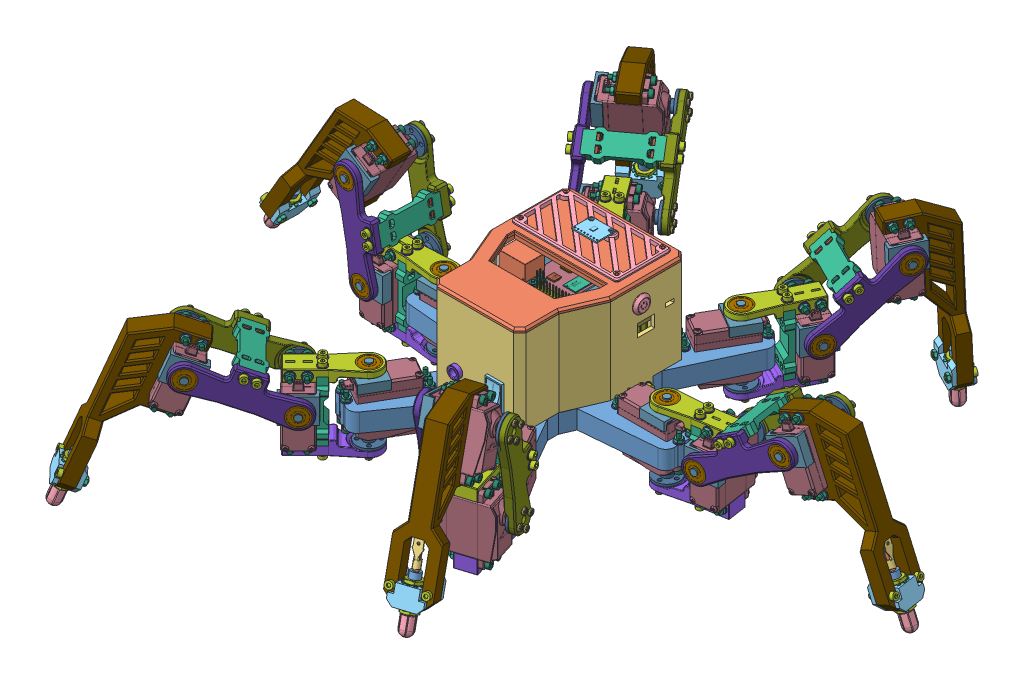
SolidWorks assembly HEXUMI_DSSERVO, configuration Default. Lengths in mm.
Overall size (517.79 216.76 502.75).
850 component instances, 62 part files, 169 mates.
Components (placement in the parent):
- BODY_ASM-1: BODY_ASM [Default] at origin size (216.8 93.6 230.48)
  - MAIN_FRAME-1: MAIN_FRAME [Default] at origin size (216.8 15 230.48)
  - LID-1: LID [Default] at (-25.1298 69 304.4932) x (1 0 0) z (0 1 0) size (97 123 7)
  - MID CASE-1: MID CASE [Default] at origin size (97 79 123)
  - ON_SWITCH-1: ON_SWITCH [Default] at (33.5 56 5) x (0 0.109318 -0.994007) z (0 -0.994007 -0.109318) size (13.7 18.1 13.7)
  - POWER_SWITCH-1: POWER_SWITCH [Default] at (16.5 19.5 76) x (0 -1 0) z (-1 0 0) size (20.5 20.17 13.5)
  - M3_HEX_NUT-1: M3_HEX_NUT [Default] at (-35 -5 0) x (0 -0.865861 0.500284) z (0 0.500284 0.865861) size (6.98 2.4 5.5)
  - M3_STEEL_HEX_BOLT_16MM-1: M3_STEEL_HEX_BOLT_16MM [Default] at (0 -5 -36.5) x (0.06898 0.997618 0) z (0.997618 -0.06898 0) size (5.68 19 5.68)
  - M3_WASHER-1: M3_WASHER [Default] at (-49 -5 0) x (0 -0.533756 -0.845639) z (0 -0.845639 0.533756) size (7 0.5 7)
  - M3_HEX_NUT-2: M3_HEX_NUT [Default] at (0 -5 -20.5) x (0.938223 0.346031 0) z (0.346031 -0.938223 0) size (6.98 2.4 5.5)
  - M3_HEX_NUT-3: M3_HEX_NUT [Default] at (0 -5 75.1) x (0.997389 -0.072217 0) z (-0.072217 -0.997389 0) size (6.98 2.4 5.5)
  - M3_HEX_NUT-4: M3_HEX_NUT [Default] at (32.6 -5 0) x (0 -0.520946 -0.85359) z (0 -0.85359 0.520946) size (6.98 2.4 5.5)
  - M3_STEEL_HEX_BOLT_16MM-2: M3_STEEL_HEX_BOLT_16MM [Default] at (-52 -5 0) x (0 -0.536208 -0.844086) z (0 -0.844086 0.536208) size (5.68 19 5.68)
  - M3_STEEL_HEX_BOLT_16MM-3: M3_STEEL_HEX_BOLT_16MM [Default] at (52 -5 0) x (0 0.249062 -0.968488) z (0 0.968488 0.249062) size (5.68 19 5.68)
  - M3_STEEL_HEX_BOLT_16MM-4: M3_STEEL_HEX_BOLT_16MM [Default] at (0 -5 93.5) x (-0.010084 0.999949 0) z (-0.999949 -0.010084 0) size (5.68 19 5.68)
  - M3_WASHER-2: M3_WASHER [Default] at (48.5 -5 0) x (0 -0.753455 -0.657499) z (0 -0.657499 0.753455) size (7 0.5 7)
  - M3_WASHER-3: M3_WASHER [Default] at (0 -5 90.5) x (0.583401 0.812184 0) z (-0.812184 0.583401 0) size (7 0.5 7)
  - M3_WASHER-4: M3_WASHER [Default] at (0 -5 -33) x (0.7999 0.600134 0) z (-0.600134 0.7999 0) size (7 0.5 7)
  - INNER_FRAME_ASM_BRASS-1: INNER_FRAME_ASM_BRASS [Default] at (0 3.6 0) size (89.3 62.14 116.59)
    - power frame R-1: power frame R [Default] at origin size (85 4 113)
    - M2.5_STEEL_HEX_NUT-1: M2.5_STEEL_HEX_NUT [Default] at (39 -1.8 -24.5) x (-0.53176 0 -0.846895) z (0.846895 0 -0.53176) size (6.22 1.8 4.9)
    - M2.5_STEEL_HEX_NUT-2: M2.5_STEEL_HEX_NUT [Default] at (-28.3 -1.8 82.3) x (-0.926596 0 0.376059) z (-0.376059 0 -0.926596) size (6.22 1.8 4.9)
    - M2.5_STEEL_HEX_NUT-3: M2.5_STEEL_HEX_NUT [Default] at (28.3 -1.8 82.3) x (-0.90596 0 -0.423363) z (0.423363 0 -0.90596) size (6.22 1.8 4.9)
    - M2.5_STEEL_HEX_NUT-4: M2.5_STEEL_HEX_NUT [Default] at (-19 -1.8 -24.5) x (0.987479 0 -0.157753) z (0.157753 0 0.987479) size (6.22 1.8 4.9)
    - M2.5_BRASS_SPACER_20MM-1: M2.5_BRASS_SPACER_20MM [Default] at (28.3 16.5 82.3) x (0.147579 0 -0.98905) z (0.98905 0 0.147579) size (5.43 25 4.7)
    - M2.5_BRASS_SPACER_20MM-2: M2.5_BRASS_SPACER_20MM [Default] at (-19 16.5 -24.5) x (0.999419 0 0.034097) z (-0.034097 0 0.999419) size (5.43 25 4.7)
    - M2.5_BRASS_SPACER_20MM-3: M2.5_BRASS_SPACER_20MM [Default] at (-28.3 16.5 82.3) x (0.586169 0 0.810189) z (-0.810189 0 0.586169) size (5.43 25 4.7)
    - M2.5_BRASS_SPACER_20MM-4: M2.5_BRASS_SPACER_20MM [Default] at (39 16.5 -24.5) x (0.00416 0 -0.999991) z (0.999991 0 0.00416) size (5.43 25 4.7)
    - RPi FRAME-1: RPi FRAME [Default] at (0 30.8 0) size (85 4 113)
    - M2.5_STEEL_HEX_NUT-9: M2.5_STEEL_HEX_NUT [Default] at (39 34.8 -24.5) x (0.941663 0 -0.336557) z (0.336557 0 0.941663) size (6.22 1.8 4.9)
    - M2.5_STEEL_HEX_NUT-10: M2.5_STEEL_HEX_NUT [Default] at (28.3 34.8 82.3) x (-0.299428 0 -0.954119) z (0.954119 0 -0.299428) size (6.22 1.8 4.9)
    - M2.5_STEEL_HEX_NUT-11: M2.5_STEEL_HEX_NUT [Default] at (28.3 34.8 45.7) x (-0.609973 0 0.792422) z (-0.792422 0 -0.609973) size (6.22 1.8 4.9)
    - M2.5_STEEL_HEX_NUT-12: M2.5_STEEL_HEX_NUT [Default] at (39 34.8 24.5) x (-0.398443 0 0.917193) z (-0.917193 0 -0.398443) size (6.22 1.8 4.9)
    - M2.5_STEEL_HEX_NUT-13: M2.5_STEEL_HEX_NUT [Default] at (-19 34.8 -24.5) x (-0.889727 0 0.456493) z (-0.456493 0 -0.889727) size (6.22 1.8 4.9)
    - M2.5_STEEL_HEX_NUT-14: M2.5_STEEL_HEX_NUT [Default] at (-19 34.8 24.5) x (-0.550521 0 -0.834821) z (0.834821 0 -0.550521) size (6.22 1.8 4.9)
    - M2.5_STEEL_HEX_NUT-15: M2.5_STEEL_HEX_NUT [Default] at (-28.3 34.8 82.3) x (-0.427939 0 0.903808) z (-0.903808 0 -0.427939) size (6.22 1.8 4.9)
    - M2.5_STEEL_HEX_NUT-16: M2.5_STEEL_HEX_NUT [Default] at (-28.3 34.8 45.7) x (-0.613101 0 -0.790005) z (0.790005 0 -0.613101) size (6.22 1.8 4.9)
    - Raspberry Pi 4 Model B-1: Raspberry Pi 4 Model B [Default] at (0 39.19 0) x (-1 0 0) z (0 0 -1) size (88.99 19.9 58.4)
      - PCB, RPi4ModelB-1: PCB, RPi4ModelB [Default] at origin size (85 1.6 56)
      - Broadcom BCM2711B0 CPU, RPi4ModelB-1: Broadcom BCM2711B0 CPU, RPi4ModelB [Default] at (-13.25 0.8 -4.5) size (15 2.3 15)
      - 2.54 mm DUPONT MALE PIN HEADER, POE, 2X2, RPi4ModelB-1: 2.54 mm DUPONT MALE PIN HEADER, POE, 2X2, RPi4ModelB [Default] at (19 0.8 -18.5) size (5.08 11.3 5.08)
      - 2.54 mm DUPONT MALE PIN HEADER, IO, 2X20, RPi4ModelB-1: 2.54 mm DUPONT MALE PIN HEADER, IO, 2X20, RPi4ModelB [Default] at (-10 0.8 -24.5) size (50.8 11.3 5.08)
      - Camera Connector, RPi4ModelB-1: Camera Connector, RPi4ModelB [Default] at (4 0.8 16.5) x (0 0 -1) z (1 0 0) size (22.4 5.68 5.07)
      - Microphone Plug, RPi4ModelB-1: Microphone Plug, RPi4ModelB [Default] at (11.5 0.8 21.65) size (7.23 7.55 15)
      - Display Connector, RPi4ModelB-1: Display Connector, RPi4ModelB [Default] at (-38.5 0.8 0) x (0 0 1) z (-1 0 0) size (22.4 5.68 5.07)
      - Gigabit Ethernet Port, RPi4ModelB-1: Gigabit Ethernet Port, RPi4ModelB [Default] at (45.5 7.55 -17.75) x (0 0 -1) z (1 0 0) size (16.2 17.24 21.64)
      - Female Micro HDMI Connector, RPi4ModelB-2: Female Micro HDMI Connector, RPi4ModelB [Default] at (-3 0.8 27.3875) size (6.5 3.51 7.5)
      - Female Micro HDMI Connector, RPi4ModelB-3: Female Micro HDMI Connector, RPi4ModelB [Default] at (-16.5 0.8 27.3875) size (6.5 3.51 7.5)
      - Female USB Type C Connector, RPi4ModelB-1: Female USB Type C Connector, RPi4ModelB [Default] at (-31.3 0.8 26.5419) size (8.94 3.96 7.9)
      - 2X USB3.0 PORTS, RPi4ModelB-2: 2X USB3.0 PORTS, RPi4ModelB [Default] at (37.07 0.8 1) size (17.47 19.41 15.68)
      - 91D77 D9WHV 778K, 4 GB LPDDR4 SDRAM, RPi4ModelB-1: 91D77 D9WHV 778K, 4 GB LPDDR4 SDRAM, RPi4ModelB [Default] at (2.25 0.8 -4.5) size (10 0.8 14.5)
      - Cypress CYW43455 Wireless Module Cover, RPi4ModelB-1: Cypress CYW43455 Wireless Module Cover, RPi4ModelB [Default] at (-30.5 0.8 -14.5) size (11 1.6 13)
      - SD Card Slot, RPi4ModelB-1: SD Card Slot, RPi4ModelB [Default] at (-35.3 -0.8 0) x (0 0 -1) z (-1 0 0) size (11.95 1.45 11.4)
      - VIA VL805 PCIe USB 3.0 controller, RPi4ModelB-1: VIA VL805 PCIe USB 3.0 controller, RPi4ModelB [Default] at (17.5 0.8 4) size (8.8 0.8 8.8)
      - 2X USB2.0 PORTS, RPi4ModelB-1: 2X USB2.0 PORTS, RPi4ModelB [Default] at (37.065 0.65 19) size (17.87 19.16 15.33)
      - Broadcom BCM54213PE Gigabit Ethernet Transceiver, RPi4ModelB-1: Broadcom BCM54213PE Gigabit Ethernet Transceiver, RPi4ModelB [Default] at (16.5 0.8 -10) size (6.8 1 6.8)
      - MxL7704 Universal PMIC, RPi4ModelB-1: MxL7704 Universal PMIC, RPi4ModelB [Default] at (-32.5 0.8 16) size (5.4 0.8 5.4)
    - M2.5_STEEL_TRI_BOLT_20MM-1: M2.5_STEEL_TRI_BOLT_20MM [Default] at (39 43.28 -24.5) x (0.010584 0 0.999944) z (0.999944 0 -0.010584) size (4.7 20 4.7)
    - M2.5_STEEL_HEX_NUT-17: M2.5_STEEL_HEX_NUT [Default] at (39 39.98 24.5) x (0.999676 0 0.025448) z (-0.025448 0 0.999676) size (6.22 1.8 4.9)
    - M2.5_STEEL_HEX_NUT-18: M2.5_STEEL_HEX_NUT [Default] at (-28.3 38.2 82.3) x (0.982697 0 -0.185221) z (0.185221 0 0.982697) size (6.22 1.8 4.9)
    - M2.5_STEEL_HEX_NUT-19: M2.5_STEEL_HEX_NUT [Default] at (28.3 38.2 82.3) size (6.22 1.8 4.9)
    - M2.5_STEEL_HEX_NUT-20: M2.5_STEEL_HEX_NUT [Default] at (28.3 38.2 45.7) size (6.22 1.8 4.9)
    - M2.5_STEEL_HEX_NUT-21: M2.5_STEEL_HEX_NUT [Default] at (-28.3 38.2 45.7) size (6.22 1.8 4.9)
    - M2.5_STEEL_HEX_NUT-22: M2.5_STEEL_HEX_NUT [Default] at (-19 39.98 24.5) x (0.99488 0 -0.101065) z (0.101065 0 0.99488) size (6.22 1.8 4.9)
    - M2.5_STEEL_HEX_NUT-23: M2.5_STEEL_HEX_NUT [Default] at (-19 39.98 -24.5) x (0.853732 0 0.520713) z (-0.520713 0 0.853732) size (6.22 1.8 4.9)
    - M2.5_STEEL_HEX_NUT-24: M2.5_STEEL_HEX_NUT [Default] at (39 39.98 -24.5) x (0.977205 0 0.212296) z (-0.212296 0 0.977205) size (6.22 1.8 4.9)
    - M2.5_STEEL_TRI_BOLT_20MM-2: M2.5_STEEL_TRI_BOLT_20MM [Default] at (28.3 41.5 82.3) x (0.000016 0 1) z (1 0 -0.000016) size (4.7 20 4.7)
    - M2.5_STEEL_TRI_BOLT_20MM-3: M2.5_STEEL_TRI_BOLT_20MM [Default] at (-28.3 41.5 82.3) x (0.000016 0 1) z (1 0 -0.000016) size (4.7 20 4.7)
    - M2.5_STEEL_TRI_BOLT_20MM-4: M2.5_STEEL_TRI_BOLT_20MM [Default] at (-19 43.28 -24.5) x (0.000016 0 1) z (1 0 -0.000016) size (4.7 20 4.7)
    - SERVO_2040-1: SERVO_2040 [Default] at (0 36.6 64) x (-1 0 0) z (0 0 -1) size (63.5 10.6 42)
    - M2.5_NYLON_BOLT-1: M2.5_NYLON_BOLT [Default] at (-28.3 41.5 45.7) x (0.149804 0 0.988716) z (0.988716 0 -0.149804) size (4.7 15 4.7)
    - M2.5_NYLON_BOLT-2: M2.5_NYLON_BOLT [Default] at (39 43.28 24.5) x (0.149804 0 0.988716) z (0.988716 0 -0.149804) size (4.7 15 4.7)
    - M2.5_NYLON_BOLT-3: M2.5_NYLON_BOLT [Default] at (28.3 41.5 45.7) x (0.149804 0 0.988716) z (0.988716 0 -0.149804) size (4.7 15 4.7)
    - M2.5_NYLON_BOLT-4: M2.5_NYLON_BOLT [Default] at (-19 43.28 24.5) x (0.05042 0 -0.998728) z (-0.998728 0 -0.05042) size (4.7 15 4.7)
    - M2.5_STEEL_HEX_NUT-25: M2.5_STEEL_HEX_NUT [Default] at (28.3 29 45.7) size (6.22 1.8 4.9)
    - M2.5_STEEL_HEX_NUT-26: M2.5_STEEL_HEX_NUT [Default] at (-28.3 29 45.7) x (0.960779 0 0.277315) z (-0.277315 0 0.960779) size (6.22 1.8 4.9)
    - M2.5_STEEL_HEX_NUT-27: M2.5_STEEL_HEX_NUT [Default] at (-19 29 24.5) x (0.999926 0 0.01217) z (-0.01217 0 0.999926) size (6.22 1.8 4.9)
    - M2.5_STEEL_HEX_NUT-28: M2.5_STEEL_HEX_NUT [Default] at (39 29 24.5) x (0.999999 0 -0.001638) z (0.001638 0 0.999999) size (6.22 1.8 4.9)
    - 7V_BUCK-1: 7V_BUCK [Default] at (13.575 6 12.675) x (0 0 1) z (-1 0 0) size (65.3 21.55 50.1)
    - 3.3V_RELAY-1: 3.3V_RELAY [Default] at (-21.55 5.2 16.3) x (0 0 1) z (-1 0 0) size (70 18 17)
    - M2.5_NYLON_HEX_NUT-1: M2.5_NYLON_HEX_NUT [Default] at (0.65 -2 41.35) size (5.66 2 4.9)
    - M2.5_NYLON_HEX_NUT-2: M2.5_NYLON_HEX_NUT [Default] at (26.5 4 -16) size (5.66 2 4.9)
    - M2.5_NYLON_HEX_NUT-3: M2.5_NYLON_HEX_NUT [Default] at (0.65 4 41.35) size (5.66 2 4.9)
    - M2.5_NYLON_HEX_NUT-4: M2.5_NYLON_HEX_NUT [Default] at (26.5 -2 41.35) size (5.66 2 4.9)
    - M2.5_NYLON_HEX_NUT-5: M2.5_NYLON_HEX_NUT [Default] at (26.5 4 41.35) size (5.66 2 4.9)
    - M2.5_NYLON_HEX_NUT-6: M2.5_NYLON_HEX_NUT [Default] at (0.65 4 -16) size (5.66 2 4.9)
    - M2.5_NYLON_HEX_NUT-7: M2.5_NYLON_HEX_NUT [Default] at (0.65 -2 -16) size (5.66 2 4.9)
    - M2.5_NYLON_HEX_NUT-8: M2.5_NYLON_HEX_NUT [Default] at (26.5 -2 -16) size (5.66 2 4.9)
    - M2_NYLON_HEX_NUT-1: M2_NYLON_HEX_NUT [Default] at (-27.75 4 -16) size (4.39 1.2 3.8)
    - M2_NYLON_HEX_NUT-2: M2_NYLON_HEX_NUT [Default] at (-27.75 -1.2 48.6) x (0.996977 0 0.0777) z (-0.0777 0 0.996977) size (4.39 1.2 3.8)
    - M2_NYLON_HEX_NUT-3: M2_NYLON_HEX_NUT [Default] at (-15.35 4 -16) size (4.39 1.2 3.8)
    - M2_NYLON_HEX_NUT-5: M2_NYLON_HEX_NUT [Default] at (-15.35 -1.2 48.6) size (4.39 1.2 3.8)
    - M2_NYLON_HEX_NUT-6: M2_NYLON_HEX_NUT [Default] at (-15.35 -1.2 -16) x (-0.796408 0 -0.604759) z (0.604759 0 -0.796408) size (4.39 1.2 3.8)
    - M2_NYLON_HEX_NUT-8: M2_NYLON_HEX_NUT [Default] at (-27.75 -1.2 -16) x (-0.852858 0 0.522143) z (-0.522143 0 -0.852858) size (4.39 1.2 3.8)
    - M2_NYLON_HEX_NUT-9: M2_NYLON_HEX_NUT [Default] at (-27.75 4 48.6) size (4.39 1.2 3.8)
    - M2_NYLON_HEX_NUT-10: M2_NYLON_HEX_NUT [Default] at (-15.35 4 48.6) size (4.39 1.2 3.8)
    - M2.5_STEEL_HEX_NUT-29: M2.5_STEEL_HEX_NUT [Default] at (-28.3 29 82.3) x (-0.398443 0 0.917193) z (-0.917193 0 -0.398443) size (6.22 1.8 4.9)
    - M2.5_STEEL_HEX_NUT-30: M2.5_STEEL_HEX_NUT [Default] at (-19 29 -24.5) x (-0.398443 0 0.917193) z (-0.917193 0 -0.398443) size (6.22 1.8 4.9)
    - M2.5_STEEL_HEX_NUT-31: M2.5_STEEL_HEX_NUT [Default] at (28.3 29 82.3) x (-0.187174 0 0.982327) z (-0.982327 0 -0.187174) size (6.22 1.8 4.9)
    - M2.5_STEEL_HEX_NUT-32: M2.5_STEEL_HEX_NUT [Default] at (39 29 -24.5) x (-0.432758 0 0.90151) z (-0.90151 0 -0.432758) size (6.22 1.8 4.9)
    - M2.5_NYLON_BOLT-5: M2.5_NYLON_BOLT [Default] at (26.5 9.05 41.35) x (0.298465 0 -0.954421) z (-0.954421 0 -0.298465) size (4.7 15 4.7)
    - M2.5_NYLON_BOLT-6: M2.5_NYLON_BOLT [Default] at (0.65 9.05 -16) x (0.311969 0 -0.950092) z (-0.950092 0 -0.311969) size (4.7 15 4.7)
    - M2.5_NYLON_BOLT-7: M2.5_NYLON_BOLT [Default] at (26.5 9.05 -16) x (0.298465 0 -0.954421) z (-0.954421 0 -0.298465) size (4.7 15 4.7)
    - M2.5_NYLON_BOLT-8: M2.5_NYLON_BOLT [Default] at (0.65 9.05 41.35) x (0.298465 0 -0.954421) z (-0.954421 0 -0.298465) size (4.7 15 4.7)
    - M2_NYLON_BOLT-1: M2_NYLON_BOLT [Default] at (-27.75 7.8 48.6) x (-0.556663 0 -0.830738) z (-0.830738 0 0.556663) size (3.8 10 3.8)
    - M2_NYLON_BOLT-2: M2_NYLON_BOLT [Default] at (-15.35 7.8 48.6) x (-0.518121 0 -0.855307) z (-0.855307 0 0.518121) size (3.8 10 3.8)
    - M2_NYLON_BOLT-3: M2_NYLON_BOLT [Default] at (-27.75 7.8 -16) x (-0.556663 0 -0.830738) z (-0.830738 0 0.556663) size (3.8 10 3.8)
    - M2_NYLON_BOLT-4: M2_NYLON_BOLT [Default] at (-15.35 7.8 -16) x (-0.556663 0 -0.830738) z (-0.830738 0 0.556663) size (3.8 10 3.8)
    - 5v_buck-1: 5v_buck [Default] at (19 31.6 -14) x (1 0 0) z (0 0 -1) size (33 7.8 28.5)
    - M2_NYLON_BOLT-5: M2_NYLON_BOLT [Default] at (32.95 35.9 -15.7) x (0.89104 0 -0.453925) z (-0.453925 0 -0.89104) size (3.8 10 3.8)
    - M2_NYLON_BOLT-6: M2_NYLON_BOLT [Default] at (5.05 35.9 -2.5) x (0.891706 0 -0.452615) z (-0.452615 0 -0.891706) size (3.8 10 3.8)
    - M2_NYLON_BOLT-7: M2_NYLON_BOLT [Default] at (5.05 35.9 -15.7) x (0.896031 0 -0.443992) z (-0.443992 0 -0.896031) size (3.8 10 3.8)
    - M2_NYLON_BOLT-8: M2_NYLON_BOLT [Default] at (32.95 35.9 -2.5) x (0.891706 0 -0.452615) z (-0.452615 0 -0.891706) size (3.8 10 3.8)
    - M2_NYLON_HEX_NUT-11: M2_NYLON_HEX_NUT [Default] at (32.95 31.6 -2.5) size (4.39 1.2 3.8)
    - M2_NYLON_HEX_NUT-12: M2_NYLON_HEX_NUT [Default] at (32.95 31.6 -15.7) size (4.39 1.2 3.8)
    - M2_NYLON_HEX_NUT-13: M2_NYLON_HEX_NUT [Default] at (5.05 31.6 -2.5) size (4.39 1.2 3.8)
    - M2_NYLON_HEX_NUT-14: M2_NYLON_HEX_NUT [Default] at (5.05 31.6 -15.7) size (4.39 1.2 3.8)
    - M2_NYLON_HEX_NUT-15: M2_NYLON_HEX_NUT [Default] at (32.95 28.9 -15.7) size (4.39 1.2 3.8)
    - M2_NYLON_HEX_NUT-16: M2_NYLON_HEX_NUT [Default] at (5.05 28.9 -15.7) size (4.39 1.2 3.8)
    - M2_NYLON_HEX_NUT-17: M2_NYLON_HEX_NUT [Default] at (32.95 28.9 -2.5) size (4.39 1.2 3.8)
    - M2_NYLON_HEX_NUT-18: M2_NYLON_HEX_NUT [Default] at (5.05 28.9 -2.5) size (4.39 1.2 3.8)
    - M2.5_STEEL_HEX_NUT-33: M2.5_STEEL_HEX_NUT [Default] at (-19 36.6 -24.5) x (-0.398443 0 0.917193) z (-0.917193 0 -0.398443) size (6.22 1.8 4.9)
    - M2.5_STEEL_HEX_NUT-34: M2.5_STEEL_HEX_NUT [Default] at (39 36.6 24.5) x (-0.398443 0 0.917193) z (-0.917193 0 -0.398443) size (6.22 1.8 4.9)
    - M2.5_STEEL_HEX_NUT-35: M2.5_STEEL_HEX_NUT [Default] at (-19 36.6 24.5) x (-0.398443 0 0.917193) z (-0.917193 0 -0.398443) size (6.22 1.8 4.9)
    - M2.5_STEEL_HEX_NUT-36: M2.5_STEEL_HEX_NUT [Default] at (39 36.6 -24.5) x (-0.398443 0 0.917193) z (-0.917193 0 -0.398443) size (6.22 1.8 4.9)
    - M2.5_STEEL_HEX_NUT-37: M2.5_STEEL_HEX_NUT [Default] at (39 -3.6 -24.5) x (-0.586704 0 -0.809801) z (0.809801 0 -0.586704) size (6.22 1.8 4.9)
    - M2.5_STEEL_HEX_NUT-38: M2.5_STEEL_HEX_NUT [Default] at (28.3 -3.6 82.3) x (-0.456254 0 -0.889849) z (0.889849 0 -0.456254) size (6.22 1.8 4.9)
    - M2.5_STEEL_HEX_NUT-39: M2.5_STEEL_HEX_NUT [Default] at (-19 -3.6 -24.5) x (0.101594 0 -0.994826) z (0.994826 0 0.101594) size (6.22 1.8 4.9)
    - M2.5_STEEL_HEX_NUT-40: M2.5_STEEL_HEX_NUT [Default] at (-28.3 -3.6 82.3) x (-0.455411 0 -0.890281) z (0.890281 0 -0.455411) size (6.22 1.8 4.9)
  - M2.5_STEEL_TRI_BOLT_20MM-1: M2.5_STEEL_TRI_BOLT_20MM [Default] at (-19 -8.65 -24.5) x (0.913498 0 -0.406843) z (0.406843 0 0.913498) size (4.7 20 4.7)
  - M2.5_STEEL_TRI_BOLT_20MM-2: M2.5_STEEL_TRI_BOLT_20MM [Default] at (28.3 -8.65 82.3) x (-0.766419 0 0.642341) z (-0.642341 0 -0.766419) size (4.7 20 4.7)
  - M2.5_STEEL_TRI_BOLT_20MM-3: M2.5_STEEL_TRI_BOLT_20MM [Default] at (-28.3 -8.65 82.3) x (-0.697743 0 -0.716349) z (0.716349 0 -0.697743) size (4.7 20 4.7)
  - M2.5_STEEL_TRI_BOLT_20MM-4: M2.5_STEEL_TRI_BOLT_20MM [Default] at (39 -8.65 -24.5) x (0.943102 0 -0.332503) z (0.332503 0 0.943102) size (4.7 20 4.7)
  - M2_NYLON_BOLT-1: M2_NYLON_BOLT [Default] at (38.915 77.3 -22.415) x (0.869496 0 -0.49394) z (-0.49394 0 -0.869496) size (3.8 10 3.8)
  - M2_NYLON_HEX_NUT-1: M2_NYLON_HEX_NUT [Default] at (-39.085 67.8 14.585) size (4.39 1.2 3.8)
  - M2_NYLON_HEX_NUT-2: M2_NYLON_HEX_NUT [Default] at (38.915 67.8 14.585) size (4.39 1.2 3.8)
  - M2_NYLON_HEX_NUT-3: M2_NYLON_HEX_NUT [Default] at (-39.085 67.8 -22.415) size (4.39 1.2 3.8)
  - M2_NYLON_HEX_NUT-4: M2_NYLON_HEX_NUT [Default] at (38.915 67.8 -22.415) size (4.39 1.2 3.8)
  - M2_NYLON_BOLT-2: M2_NYLON_BOLT [Default] at (-39.085 77.3 -22.415) x (0.562561 0 -0.826756) z (-0.826756 0 -0.562561) size (3.8 10 3.8)
  - M2_NYLON_BOLT-3: M2_NYLON_BOLT [Default] at (38.915 77.3 14.585) x (0.001977 0 -0.999998) z (-0.999998 0 -0.001977) size (3.8 10 3.8)
  - M2_NYLON_BOLT-4: M2_NYLON_BOLT [Default] at (-39.085 77.3 14.585) x (0.810874 0 -0.585221) z (-0.585221 0 -0.810874) size (3.8 10 3.8)
  - M2_NYLON_HEX_NUT-5: M2_NYLON_HEX_NUT [Default] at (-39.085 72 -22.415) x (0.987617 0 -0.156887) z (0.156887 0 0.987617) size (4.39 1.2 3.8)
  - M2_NYLON_HEX_NUT-6: M2_NYLON_HEX_NUT [Default] at (-39.085 72 14.585) x (0.982983 0 0.183699) z (-0.183699 0 0.982983) size (4.39 1.2 3.8)
  - M2_NYLON_HEX_NUT-7: M2_NYLON_HEX_NUT [Default] at (38.915 72 14.585) x (0.858157 0 0.513388) z (-0.513388 0 0.858157) size (4.39 1.2 3.8) (hidden)
  - M2_NYLON_HEX_NUT-8: M2_NYLON_HEX_NUT [Default] at (38.915 72 -22.415) x (0.965887 0 0.258962) z (-0.258962 0 0.965887) size (4.39 1.2 3.8)
  - MPU6050_STAND-3: MPU6050_STAND [Default] at (-0.085 73.2 -3.915) x (-1 0 0) z (0 0 -1) size (86 4 45)
  - Gyroscope sensor-1: Gyroscope sensor [Default] at (-0.085 77.2 -5.915) x (0 0 -1) z (1 0 0) size (16 1.4 20)
- LEG_L-1: LEG_L [Default] at (-72.7153 -8.25 -94.0697) x (-0.804009 0 0.594617) z (0.594617 0 0.804009) size (67.5 177.4 212.11) (flexible)
  - LINK-1: LINK [Default] at origin size (20 48.5 7)
  - COXA_BEARING-1: COXA_BEARING [Default] at (0 -29.25 30) size (20 9.2 60)
  - COXA_SERVO-1: COXA_SERVO [Default] at (0 31.25 30) x (-1 0 0) z (0 0 1) size (20 11.2 60)
  - BEARING-1: BEARING [Default] at (0 -24.25 30) x (0.0625 0 0.998045) z (0 -1 0) size (16 16 5)
  - HORN-1: HORN [Default] at (0 26.25 30) x (0 0 -1) z (0 -1 0) size (20 20 4.6)
  - M3_SQUARE_NUT-1: M3_SQUARE_NUT [Default] at (-4 16.25 3.5) x (0.957271 0 -0.289193) z (0.289193 0 0.957271) size (5.3 1.7 5.3)
  - M3_STEEL_HEX_BOLT_16MM-1: M3_STEEL_HEX_BOLT_16MM [Default] at (4 34.75 3.5) x (-0.894577 0 0.446913) z (0.446913 0 0.894577) size (5.68 19 5.68)
  - M3_WASHER-1: M3_WASHER [Default] at (4 31.25 3.5) x (0.976163 0 0.217039) z (-0.217039 0 0.976163) size (7 0.5 7)
  - M3_SERVO_HORN_BOLT-1: M3_SERVO_HORN_BOLT [Default] at (-7 33.25 30) x (-0.783548 0 -0.621331) z (-0.621331 0 0.783548) size (4.8 7 4.8)
  - M3_SERVO_HORN_BOLT-2: M3_SERVO_HORN_BOLT [Default] at (7 33.25 30) x (-0.783548 0 -0.621331) z (-0.621331 0 0.783548) size (4.8 7 4.8)
  - M3_SERVO_HORN_BOLT-3: M3_SERVO_HORN_BOLT [Default] at (0 33.25 37) x (-0.783548 0 -0.621331) z (-0.621331 0 0.783548) size (4.8 7 4.8)
  - M3_SERVO_HORN_BOLT-4: M3_SERVO_HORN_BOLT [Default] at (0 33.25 23) x (-0.783548 0 -0.621331) z (-0.621331 0 0.783548) size (4.8 7 4.8)
  - M3_SQUARE_NUT-2: M3_SQUARE_NUT [Default] at (4 16.25 3.5) x (0.957271 0 -0.289193) z (0.289193 0 0.957271) size (5.3 1.7 5.3)
  - M3_SQUARE_NUT-3: M3_SQUARE_NUT [Default] at (-4 -15.95 3.5) x (0.957271 0 -0.289193) z (0.289193 0 0.957271) size (5.3 1.7 5.3)
  - M3_SQUARE_NUT-4: M3_SQUARE_NUT [Default] at (4 -15.95 3.5) x (0.957271 0 -0.289193) z (0.289193 0 0.957271) size (5.3 1.7 5.3)
  - M3_STEEL_HEX_BOLT_16MM-2: M3_STEEL_HEX_BOLT_16MM [Default] at (-4 -32.75 3.5) x (0.957271 0 -0.289193) z (0.289193 0 0.957271) size (5.68 19 5.68)
  - M3_STEEL_HEX_BOLT_16MM-3: M3_STEEL_HEX_BOLT_16MM [Default] at (4 -32.75 3.5) x (0.957271 0 -0.289193) z (0.289193 0 0.957271) size (5.68 19 5.68)
  - M3_STEEL_HEX_BOLT_16MM-4: M3_STEEL_HEX_BOLT_16MM [Default] at (-4 34.75 3.5) x (-0.774913 0 0.632068) z (0.632068 0 0.774913) size (5.68 19 5.68)
  - M3_WASHER-2: M3_WASHER [Default] at (4 -29.75 3.5) x (0.951621 0 -0.307274) z (0.307274 0 0.951621) size (7 0.5 7)
  - M3_WASHER-3: M3_WASHER [Default] at (-4 -29.75 3.5) x (0.857471 0 -0.514532) z (0.514532 0 0.857471) size (7 0.5 7)
  - M3_WASHER-4: M3_WASHER [Default] at (-4 31.25 3.5) x (0.999494 0 -0.031797) z (0.031797 0 0.999494) size (7 0.5 7)
  - SERVO_ASM-1: SERVO_ASM [Default] at (-25.8 -9.95 -10.2) x (0 1 0) z (-1 0 0) size (87.25 24.4 54.8)
    - SW2020 DS3225MG Servo 25Kg 4.8-6.8V-2: SW2020 DS3225MG Servo 25Kg 4.8-6.8V [Default] at origin size (54.3 20.4 45.91)
    - SERVO_CLIP-1: SERVO_CLIP [Default] at (0 0 -45.6) x (-1 0 0) z (0 0 -1) size (20 24.4 14.2)
  - SERVO_ASM-2: SERVO_ASM [Default] at (0 24.55 30) x (0.112948 0 0.993601) z (0 1 0) size (87.25 24.4 54.8)
    - SW2020 DS3225MG Servo 25Kg 4.8-6.8V-2: SW2020 DS3225MG Servo 25Kg 4.8-6.8V [Default] at origin size (54.3 20.4 45.91)
    - SERVO_CLIP-1: SERVO_CLIP [Default] at (0 0 -45.6) x (-1 0 0) z (0 0 -1) size (20 24.4 14.2)
  - M3_HEX_NUT-1: M3_HEX_NUT [Default] at (10.4 -24.75 -15.2) x (0 0.554401 -0.83225) z (0 0.83225 0.554401) size (6.98 2.4 5.5)
  - M3_SQUARE_NUT-5: M3_SQUARE_NUT [Default] at (0.85 24.85 -15.2) x (0 0 -1) z (0 1 0) size (5.3 1.7 5.3)
  - M3_STEEL_HEX_BOLT-1: M3_STEEL_HEX_BOLT [Default] at (-14.2 -24.75 -5.2) x (0 -0.390994 0.920393) z (0 0.920393 0.390994) size (5.68 28 5.68)
  - M3_WASHER-5: M3_WASHER [Default] at (8 -24.75 -5.2) x (0 -0.313666 0.949533) z (0 0.949533 0.313666) size (7 0.5 7)
  - M3_WASHER-6: M3_WASHER [Default] at (8 -24.75 -15.2) x (0 -0.313666 0.949533) z (0 0.949533 0.313666) size (7 0.5 7)
  - M3_WASHER-7: M3_WASHER [Default] at (8 24.85 -15.2) x (0 -0.313666 0.949533) z (0 0.949533 0.313666) size (7 0.5 7)
  - M3_WASHER-8: M3_WASHER [Default] at (8 24.85 -5.2) x (0 -0.313666 0.949533) z (0 0.949533 0.313666) size (7 0.5 7)
  - M3_STEEL_HEX_BOLT-2: M3_STEEL_HEX_BOLT [Default] at (-14.2 24.85 -15.2) x (0 -0.835258 0.549858) z (0 0.549858 0.835258) size (5.68 28 5.68)
  - M3_STEEL_HEX_BOLT-3: M3_STEEL_HEX_BOLT [Default] at (-14.2 -24.75 -15.2) x (0 0.230066 0.973175) z (0 0.973175 -0.230066) size (5.68 28 5.68)
  - M3_STEEL_HEX_BOLT-4: M3_STEEL_HEX_BOLT [Default] at (-14.2 24.85 -5.2) x (0 -0.984641 0.17459) z (0 0.17459 0.984641) size (5.68 28 5.68)
  - M3_SQUARE_NUT-6: M3_SQUARE_NUT [Default] at (0.85 -24.75 -5.2) x (0 1 0) z (0 0 1) size (5.3 1.7 5.3)
  - M3_SQUARE_NUT-7: M3_SQUARE_NUT [Default] at (0.85 -24.75 -15.2) x (0 1 0) z (0 0 1) size (5.3 1.7 5.3)
  - M3_SQUARE_NUT-8: M3_SQUARE_NUT [Default] at (0.85 24.85 -5.2) x (0 0 -1) z (0 1 0) size (5.3 1.7 5.3)
  - M3_HEX_NUT-2: M3_HEX_NUT [Default] at (10.4 -24.75 -5.2) x (0 0.450627 -0.892712) z (0 0.892712 0.450627) size (6.98 2.4 5.5)
  - M3_HEX_NUT-3: M3_HEX_NUT [Default] at (10.9 24.85 -5.2) x (0 0.387589 -0.921832) z (0 0.921832 0.387589) size (6.98 2.4 5.5)
  - M3_HEX_NUT-4: M3_HEX_NUT [Default] at (10.9 24.85 -15.2) x (0 0.281781 -0.959479) z (0 0.959479 0.281781) size (6.98 2.4 5.5)
  - FEMUR_SERVO-1: FEMUR_SERVO [Default] at (-32.5 -45.5354 -70.48) x (1 0 0) z (0 -0.508363 -0.861143) size (10 28 90)
  - FEMUR_BEARING-1: FEMUR_BEARING [Default] at (28 -9.95 -10.2) x (-1 0 0) z (0 0.508363 0.861143) size (8 28 90)
  - LINK-2: LINK [Default] at (-1.25 -43.2433 -31.1895) x (0 -0.508363 -0.861143) z (0 0.861143 -0.508363) size (20 48.5 7)
  - BEARING-2: BEARING [Default] at (28 -9.95 -10.2) x (0 0.418384 0.90827) z (-1 0 0) size (16 16 5)
  - HORN-2: HORN [Default] at (-27.5 -9.95 -10.2) x (0 -0.861143 0.508363) z (1 0 0) size (20 20 4.6)
  - BEARING-3: BEARING [Default] at (28 -45.5354 -70.48) x (0 0.418384 0.90827) z (-1 0 0) size (16 16 5)
  - HORN-3: HORN [Default] at (-27.5 -45.5354 -70.48) x (0 0.508363 0.861143) z (1 0 0) size (20 20 4.6)
  - M3_HEX_NUT-5: M3_HEX_NUT [Default] at (8.5 -10.5203 -73.6393) x (0 -0.996607 0.082307) z (0 0.082307 0.996607) size (6.98 2.4 5.5)
  - M3_SERVO_HORN_BOLT-5: M3_SERVO_HORN_BOLT [Default] at (-34.5 -15.978 -6.6415) x (0 0.998165 -0.060547) z (0 -0.060547 -0.998165) size (4.8 7 4.8)
  - M3_SQUARE_NUT-9: M3_SQUARE_NUT [Default] at (-17.5 -38.1958 -29.5242) x (0 0.508363 0.861143) z (0 -0.861143 0.508363) size (5.3 1.7 5.3)
  - M3_STEEL_HEX_BOLT-5: M3_STEEL_HEX_BOLT [Default] at (-14.2 -61.0895 -71.9325) x (0 -0.933228 -0.359286) z (0 -0.359286 0.933228) size (5.68 28 5.68)
  - M3_STEEL_HEX_BOLT_16MM-5: M3_STEEL_HEX_BOLT_16MM [Default] at (31.5 -38.1958 -29.5242) x (0 0.963892 0.266294) z (0 -0.266294 0.963892) size (5.68 19 5.68)
  - M3_WASHER-9: M3_WASHER [Default] at (28.5 -38.1958 -29.5242) x (0 0.36047 0.932771) z (0 -0.932771 0.36047) size (7 0.5 7)
  - M3_SERVO_HORN_BOLT-6: M3_SERVO_HORN_BOLT [Default] at (-34.5 -3.922 -13.7585) x (0 0.373361 -0.927686) z (0 -0.927686 -0.373361) size (4.8 7 4.8)
  - M3_SERVO_HORN_BOLT-7: M3_SERVO_HORN_BOLT [Default] at (-34.5 -41.9768 -64.452) x (0 0.325507 -0.94554) z (0 -0.94554 -0.325507) size (4.8 7 4.8)
  - M3_SERVO_HORN_BOLT-8: M3_SERVO_HORN_BOLT [Default] at (-34.5 -39.5074 -74.0386) x (0 0.184546 -0.982824) z (0 -0.982824 -0.184546) size (4.8 7 4.8)
  - M3_SERVO_HORN_BOLT-9: M3_SERVO_HORN_BOLT [Default] at (-34.5 -51.5634 -66.9215) x (0 0.681327 -0.731979) z (0 -0.731979 -0.681327) size (4.8 7 4.8)
  - M3_SERVO_HORN_BOLT-10: M3_SERVO_HORN_BOLT [Default] at (-34.5 -49.0939 -76.508) x (0 0.520293 -0.853988) z (0 -0.853988 -0.520293) size (4.8 7 4.8)
  - M3_SERVO_HORN_BOLT-11: M3_SERVO_HORN_BOLT [Default] at (-34.5 -6.3915 -4.172) x (0 -0.171182 -0.985239) z (0 -0.985239 0.171182) size (4.8 7 4.8)
  - M3_SERVO_HORN_BOLT-12: M3_SERVO_HORN_BOLT [Default] at (-34.5 -13.5085 -16.228) x (0 0.672311 -0.740269) z (0 -0.740269 -0.672311) size (4.8 7 4.8)
  - M3_SERVO_HORN_BOLT-13: M3_SERVO_HORN_BOLT [Default] at (-29.5 -45.5354 -70.48) x (0 0.520293 -0.853988) z (0 -0.853988 -0.520293) size (4.8 7 4.8)
  - M3_SERVO_HORN_BOLT-14: M3_SERVO_HORN_BOLT [Default] at (-29.5 -9.95 -10.2) x (0 0.520293 -0.853988) z (0 -0.853988 -0.520293) size (4.8 7 4.8)
  - M3_STEEL_HEX_BOLT_16MM-6: M3_STEEL_HEX_BOLT_16MM [Default] at (-36 -42.2627 -36.4133) x (0 -0.255744 -0.966745) z (0 -0.966745 0.255744) size (5.68 19 5.68)
  - M3_STEEL_HEX_BOLT_16MM-7: M3_STEEL_HEX_BOLT_16MM [Default] at (31.5 -42.2627 -36.4133) x (0 0.850981 0.525196) z (0 -0.525196 0.850981) size (5.68 19 5.68)
  - M3_STEEL_HEX_BOLT_16MM-8: M3_STEEL_HEX_BOLT_16MM [Default] at (-36 -38.1958 -29.5242) x (0 -0.563912 -0.825835) z (0 -0.825835 0.563912) size (5.68 19 5.68)
  - M3_WASHER-10: M3_WASHER [Default] at (28.5 -42.2627 -36.4133) x (0 0.320127 0.947375) z (0 -0.947375 0.320127) size (7 0.5 7)
  - M3_WASHER-11: M3_WASHER [Default] at (-32.5 -42.2627 -36.4133) x (0 0.222061 0.975033) z (0 -0.975033 0.222061) size (7 0.5 7)
  - M3_WASHER-12: M3_WASHER [Default] at (-32.5 -38.1958 -29.5242) x (0 0.409501 0.91231) z (0 -0.91231 0.409501) size (7 0.5 7)
  - M3_SQUARE_NUT-10: M3_SQUARE_NUT [Default] at (14.7 -42.2627 -36.4133) x (0 0.508363 0.861143) z (0 -0.861143 0.508363) size (5.3 1.7 5.3)
  - M3_SQUARE_NUT-11: M3_SQUARE_NUT [Default] at (14.7 -38.1958 -29.5242) x (0 0.508363 0.861143) z (0 -0.861143 0.508363) size (5.3 1.7 5.3)
  - M3_SQUARE_NUT-12: M3_SQUARE_NUT [Default] at (-17.5 -42.2627 -36.4133) x (0 0.508363 0.861143) z (0 -0.861143 0.508363) size (5.3 1.7 5.3)
  - SERVO_ASM-3: SERVO_ASM [Default] at (-25.8 -45.5354 -70.48) x (0 0.973051 -0.23059) z (-1 0 0) size (87.25 24.4 54.8)
    - SW2020 DS3225MG Servo 25Kg 4.8-6.8V-2: SW2020 DS3225MG Servo 25Kg 4.8-6.8V [Default] at origin size (54.3 20.4 45.91)
    - SERVO_CLIP-1: SERVO_CLIP [Default] at (0 0 -45.6) x (-1 0 0) z (0 0 -1) size (20 24.4 14.2)
  - M3_STEEL_HEX_BOLT-6: M3_STEEL_HEX_BOLT [Default] at (-14.2 -58.7836 -62.202) x (0 -0.933228 -0.359286) z (0 -0.359286 0.933228) size (5.68 28 5.68)
  - M3_STEEL_HEX_BOLT-7: M3_STEEL_HEX_BOLT [Default] at (-14.2 -10.5203 -73.6393) x (0 -0.933228 -0.359286) z (0 -0.359286 0.933228) size (5.68 28 5.68)
  - M3_STEEL_HEX_BOLT-8: M3_STEEL_HEX_BOLT [Default] at (-14.2 -12.8262 -83.3698) x (0 -0.933228 -0.359286) z (0 -0.359286 0.933228) size (5.68 28 5.68)
  - M3_WASHER-13: M3_WASHER [Default] at (8.5 -61.0895 -71.9325) x (0 -0.744989 0.667077) z (0 -0.667077 -0.744989) size (7 0.5 7)
  - M3_WASHER-14: M3_WASHER [Default] at (8.5 -10.5203 -73.6393) x (0 0.510645 0.859791) z (0 -0.859791 0.510645) size (7 0.5 7)
  - M3_WASHER-15: M3_WASHER [Default] at (8.5 -58.7836 -62.202) x (0 -0.855136 -0.518404) z (0 0.518404 -0.855136) size (7 0.5 7)
  - M3_HEX_NUT-9: M3_HEX_NUT [Default] at (8.5 -61.0895 -71.9325) x (0 -0.742673 0.669654) z (0 0.669654 0.742673) size (6.98 2.4 5.5)
  - M3_HEX_NUT-10: M3_HEX_NUT [Default] at (8.5 -58.7836 -62.202) x (0 -0.972142 0.234393) z (0 0.234393 0.972142) size (6.98 2.4 5.5)
  - M3_HEX_NUT-11: M3_HEX_NUT [Default] at (8.5 -12.8262 -83.3698) x (0 -0.862059 0.506808) z (0 0.506808 0.862059) size (6.98 2.4 5.5)
  - M3_WASHER-17: M3_WASHER [Default] at (8.5 -12.8262 -83.3698) x (0 -0.944852 -0.327497) z (0 0.327497 -0.944852) size (7 0.5 7)
  - M3_SERVO_HORN_BOLT-15: M3_SERVO_HORN_BOLT [Default] at (0 28.25 30) x (-0.080399 0 -0.996763) z (-0.996763 0 0.080399) size (4.8 7 4.8)
  - TIBIA_V2_ASM-1: TIBIA_V2_ASM [Default] at (0 -45.4266 -70.4544) x (-1 0 0) z (0 -0.973051 0.23059) size (32.11 50.6 145.7)
    - TIBIA_V2-1: TIBIA_V2 [Default] at origin size (32 47.6 127.94)
    - LIMIT_SWITCH-1: LIMIT_SWITCH [Default] at (0 32.3524 -111.7407) x (-0.992713 0.1205 0) z (0.1205 0.992713 0) size (13.8 62.3 13.8) (flexible)
      - LIMIT_SWITCH_SLEEVE-1: LIMIT_SWITCH_SLEEVE [Default] at origin size (7.7 25.25 7.7)
      - LIMIT_SWITCH_SHAFT-1: LIMIT_SWITCH_SHAFT [Default] at (0 5.5422 0) x (-0.210419 0 -0.977611) z (0.977611 0 -0.210419) size (5 52 5)
      - LIMIT_SWITCH_LIMITER-1: LIMIT_SWITCH_LIMITER [Default] at (0 26.0422 0) x (-0.600712 0 -0.799465) z (0.799465 0 -0.600712) size (6.64 21.41 7.08)
      - RUBBER_CAP-1: RUBBER_CAP [Default] at (0 -9.9578 0) x (0.575853 0 -0.817553) z (0.817553 0 0.575853) size (10 14 10)
    - FOOT_HOLD-1: FOOT_HOLD [Default] at (0 32.3524 -108.9407) x (1 0 0) z (0 -1 0) size (32 22 16)
    - LIMIT_SWITCH_WASHER-1: LIMIT_SWITCH_WASHER [Default] at (0 32.3524 -93.5407) x (0.999093 -0.042592 0) z (0.042592 0.999093 0) size (14.82 0.4 15)
    - LIMIT_SWITCH_WASHER-2: LIMIT_SWITCH_WASHER [Default] at (0 32.3524 -108.9407) x (0.999093 -0.042592 0) z (0.042592 0.999093 0) size (14.82 0.4 15)
    - LIMIT_SWITCH_NUT-1: LIMIT_SWITCH_NUT [Default] at (0 32.3524 -92.3407) x (0.997292 -0.073548 0) z (0.073548 0.997292 0) size (13.86 2.4 12)
    - LIMIT_SWITCH_NUT-2: LIMIT_SWITCH_NUT [Default] at (0 32.3524 -110.5407) x (0.999648 -0.026514 0) z (0.026514 0.999648 0) size (13.86 2.4 12)
    - M3_HEX_NUT-1: M3_HEX_NUT [Default] at (-12 21.9524 -96.9407) x (-0.996596 0 -0.082443) z (0.082443 0 -0.996596) size (6.98 2.4 5.5)
    - M3_HEX_NUT-2: M3_HEX_NUT [Default] at (12 21.9524 -96.9407) x (-0.491735 0 -0.870745) z (0.870745 0 -0.491735) size (6.98 2.4 5.5)
    - M3_STEEL_HEX_BOLT_16MM-1: M3_STEEL_HEX_BOLT_16MM [Default] at (-12 40.3524 -96.9407) x (-0.809803 0 -0.586702) z (-0.586702 0 0.809803) size (5.68 19 5.68)
    - M3_STEEL_HEX_BOLT_16MM-2: M3_STEEL_HEX_BOLT_16MM [Default] at (12 40.3524 -96.9407) x (-0.933551 0 -0.358443) z (-0.358443 0 0.933551) size (5.68 19 5.68)
- LEG_L-2: LEG_L [Default] at (-76.6324 -8.25 141.7647) x (0.700512 0 0.713641) z (0.713641 0 -0.700512) size (67.5 173.11 232.67) (flexible)
  - LINK-1: LINK [Default] at origin size (20 48.5 7)
  - COXA_BEARING-1: COXA_BEARING [Default] at (0 -29.25 30) size (20 9.2 60)
  - COXA_SERVO-1: COXA_SERVO [Default] at (0 31.25 30) x (-1 0 0) z (0 0 1) size (20 11.2 60)
  - BEARING-1: BEARING [Default] at (0 -24.25 30) x (-0.316211 0 0.948689) z (0 -1 0) size (16 16 5)
  - HORN-1: HORN [Default] at (0 26.25 30) x (0 0 -1) z (0 -1 0) size (20 20 4.6)
  - M3_SQUARE_NUT-1: M3_SQUARE_NUT [Default] at (-4 16.25 3.5) x (0.995872 0 0.090765) z (-0.090765 0 0.995872) size (5.3 1.7 5.3)
  - M3_STEEL_HEX_BOLT_16MM-1: M3_STEEL_HEX_BOLT_16MM [Default] at (4 34.75 3.5) x (-0.996878 0 0.078956) z (0.078956 0 0.996878) size (5.68 19 5.68)
  - M3_WASHER-1: M3_WASHER [Default] at (4 31.25 3.5) x (0.823608 0 0.56716) z (-0.56716 0 0.823608) size (7 0.5 7)
  - M3_SERVO_HORN_BOLT-1: M3_SERVO_HORN_BOLT [Default] at (-7 33.25 30) x (-0.493477 0 -0.869759) z (-0.869759 0 0.493477) size (4.8 7 4.8)
  - M3_SERVO_HORN_BOLT-2: M3_SERVO_HORN_BOLT [Default] at (7 33.25 30) x (-0.493477 0 -0.869759) z (-0.869759 0 0.493477) size (4.8 7 4.8)
  - M3_SERVO_HORN_BOLT-3: M3_SERVO_HORN_BOLT [Default] at (0 33.25 37) x (-0.493477 0 -0.869759) z (-0.869759 0 0.493477) size (4.8 7 4.8)
  - M3_SERVO_HORN_BOLT-4: M3_SERVO_HORN_BOLT [Default] at (0 33.25 23) x (-0.493477 0 -0.869759) z (-0.869759 0 0.493477) size (4.8 7 4.8)
  - M3_SQUARE_NUT-2: M3_SQUARE_NUT [Default] at (4 16.25 3.5) x (0.995872 0 0.090765) z (-0.090765 0 0.995872) size (5.3 1.7 5.3)
  - M3_SQUARE_NUT-3: M3_SQUARE_NUT [Default] at (-4 -15.95 3.5) x (0.995872 0 0.090765) z (-0.090765 0 0.995872) size (5.3 1.7 5.3)
  - M3_SQUARE_NUT-4: M3_SQUARE_NUT [Default] at (4 -15.95 3.5) x (0.995872 0 0.090765) z (-0.090765 0 0.995872) size (5.3 1.7 5.3)
  - M3_STEEL_HEX_BOLT_16MM-2: M3_STEEL_HEX_BOLT_16MM [Default] at (-4 -32.75 3.5) x (0.995872 0 0.090765) z (-0.090765 0 0.995872) size (5.68 19 5.68)
  - M3_STEEL_HEX_BOLT_16MM-3: M3_STEEL_HEX_BOLT_16MM [Default] at (4 -32.75 3.5) x (0.995872 0 0.090765) z (-0.090765 0 0.995872) size (5.68 19 5.68)
  - M3_STEEL_HEX_BOLT_16MM-4: M3_STEEL_HEX_BOLT_16MM [Default] at (-4 34.75 3.5) x (-0.955353 0 0.295468) z (0.295468 0 0.955353) size (5.68 19 5.68)
  - M3_WASHER-2: M3_WASHER [Default] at (4 -29.75 3.5) x (0.997413 0 0.071884) z (-0.071884 0 0.997413) size (7 0.5 7)
  - M3_WASHER-3: M3_WASHER [Default] at (-4 -29.75 3.5) x (0.987827 0 -0.155555) z (0.155555 0 0.987827) size (7 0.5 7)
  - M3_WASHER-4: M3_WASHER [Default] at (-4 31.25 3.5) x (0.938523 0 0.345218) z (-0.345218 0 0.938523) size (7 0.5 7)
  - SERVO_ASM-1: SERVO_ASM [Default] at (-25.8 -9.95 -10.2) x (0 1 0) z (-1 0 0) size (87.25 24.4 54.8)
    - SW2020 DS3225MG Servo 25Kg 4.8-6.8V-2: SW2020 DS3225MG Servo 25Kg 4.8-6.8V [Default] at origin size (54.3 20.4 45.91)
    - SERVO_CLIP-1: SERVO_CLIP [Default] at (0 0 -45.6) x (-1 0 0) z (0 0 -1) size (20 24.4 14.2)
  - SERVO_ASM-2: SERVO_ASM [Default] at (0 24.55 30) x (-0.267775 0 0.963481) z (0 1 0) size (87.25 24.4 54.8)
    - SW2020 DS3225MG Servo 25Kg 4.8-6.8V-2: SW2020 DS3225MG Servo 25Kg 4.8-6.8V [Default] at origin size (54.3 20.4 45.91)
    - SERVO_CLIP-1: SERVO_CLIP [Default] at (0 0 -45.6) x (-1 0 0) z (0 0 -1) size (20 24.4 14.2)
  - M3_HEX_NUT-1: M3_HEX_NUT [Default] at (10.4 -24.75 -15.2) x (0 0.554401 -0.83225) z (0 0.83225 0.554401) size (6.98 2.4 5.5)
  - M3_SQUARE_NUT-5: M3_SQUARE_NUT [Default] at (0.85 24.85 -15.2) x (0 0 -1) z (0 1 0) size (5.3 1.7 5.3)
  - M3_STEEL_HEX_BOLT-1: M3_STEEL_HEX_BOLT [Default] at (-14.2 -24.75 -5.2) x (0 -0.390994 0.920393) z (0 0.920393 0.390994) size (5.68 28 5.68)
  - M3_WASHER-5: M3_WASHER [Default] at (8 -24.75 -5.2) x (0 -0.313666 0.949533) z (0 0.949533 0.313666) size (7 0.5 7)
  - M3_WASHER-6: M3_WASHER [Default] at (8 -24.75 -15.2) x (0 -0.313666 0.949533) z (0 0.949533 0.313666) size (7 0.5 7)
  - M3_WASHER-7: M3_WASHER [Default] at (8 24.85 -15.2) x (0 -0.313666 0.949533) z (0 0.949533 0.313666) size (7 0.5 7)
  - M3_WASHER-8: M3_WASHER [Default] at (8 24.85 -5.2) x (0 -0.313666 0.949533) z (0 0.949533 0.313666) size (7 0.5 7)
  - M3_STEEL_HEX_BOLT-2: M3_STEEL_HEX_BOLT [Default] at (-14.2 24.85 -15.2) x (0 -0.835258 0.549858) z (0 0.549858 0.835258) size (5.68 28 5.68)
  - M3_STEEL_HEX_BOLT-3: M3_STEEL_HEX_BOLT [Default] at (-14.2 -24.75 -15.2) x (0 0.230066 0.973175) z (0 0.973175 -0.230066) size (5.68 28 5.68)
  - M3_STEEL_HEX_BOLT-4: M3_STEEL_HEX_BOLT [Default] at (-14.2 24.85 -5.2) x (0 -0.984641 0.17459) z (0 0.17459 0.984641) size (5.68 28 5.68)
  - M3_SQUARE_NUT-6: M3_SQUARE_NUT [Default] at (0.85 -24.75 -5.2) x (0 1 0) z (0 0 1) size (5.3 1.7 5.3)
  - M3_SQUARE_NUT-7: M3_SQUARE_NUT [Default] at (0.85 -24.75 -15.2) x (0 1 0) z (0 0 1) size (5.3 1.7 5.3)
  - M3_SQUARE_NUT-8: M3_SQUARE_NUT [Default] at (0.85 24.85 -5.2) x (0 0 -1) z (0 1 0) size (5.3 1.7 5.3)
  - M3_HEX_NUT-2: M3_HEX_NUT [Default] at (10.4 -24.75 -5.2) x (0 0.450627 -0.892712) z (0 0.892712 0.450627) size (6.98 2.4 5.5)
  - M3_HEX_NUT-3: M3_HEX_NUT [Default] at (10.9 24.85 -5.2) x (0 0.387589 -0.921832) z (0 0.921832 0.387589) size (6.98 2.4 5.5)
  - M3_HEX_NUT-4: M3_HEX_NUT [Default] at (10.9 24.85 -15.2) x (0 0.281781 -0.959479) z (0 0.959479 0.281781) size (6.98 2.4 5.5)
  - FEMUR_SERVO-1: FEMUR_SERVO [Default] at (-32.5 -35.3838 -75.416) x (1 0 0) z (0 -0.36334 -0.931657) size (10 28 90)
  - FEMUR_BEARING-1: FEMUR_BEARING [Default] at (28 -9.95 -10.2) x (-1 0 0) z (0 0.36334 0.931657) size (8 28 90)
  - LINK-2: LINK [Default] at (-1.25 -39.4367 -36.2679) x (0 -0.36334 -0.931657) z (0 0.931657 -0.36334) size (20 48.5 7)
  - BEARING-2: BEARING [Default] at (28 -9.95 -10.2) x (0 0.418384 0.90827) z (-1 0 0) size (16 16 5)
  - HORN-2: HORN [Default] at (-27.5 -9.95 -10.2) x (0 -0.931657 0.36334) z (1 0 0) size (20 20 4.6)
  - BEARING-3: BEARING [Default] at (28 -35.3838 -75.416) x (0 0.418384 0.90827) z (-1 0 0) size (16 16 5)
  - HORN-3: HORN [Default] at (-27.5 -35.3838 -75.416) x (0 0.36334 0.931657) z (1 0 0) size (20 20 4.6)
  - M3_HEX_NUT-5: M3_HEX_NUT [Default] at (8.5 -1.1366 -83.3637) x (0 -0.996607 0.082307) z (0 0.082307 0.996607) size (6.98 2.4 5.5)
  - M3_SERVO_HORN_BOLT-5: M3_SERVO_HORN_BOLT [Default] at (-34.5 -16.4716 -7.6566) x (0 0.998165 -0.060547) z (0 -0.060547 -0.998165) size (4.8 7 4.8)
  - M3_SQUARE_NUT-9: M3_SQUARE_NUT [Default] at (-17.5 -34.7226 -33.8129) x (0 0.36334 0.931657) z (0 -0.931657 0.36334) size (5.3 1.7 5.3)
  - M3_STEEL_HEX_BOLT-5: M3_STEEL_HEX_BOLT [Default] at (-14.2 -50.9898 -74.7142) x (0 -0.933228 -0.359286) z (0 -0.359286 0.933228) size (5.68 28 5.68)
  - M3_STEEL_HEX_BOLT_16MM-5: M3_STEEL_HEX_BOLT_16MM [Default] at (31.5 -34.7226 -33.8129) x (0 0.963892 0.266294) z (0 -0.266294 0.963892) size (5.68 19 5.68)
  - M3_WASHER-9: M3_WASHER [Default] at (28.5 -34.7226 -33.8129) x (0 0.36047 0.932771) z (0 -0.932771 0.36047) size (7 0.5 7)
  - M3_SERVO_HORN_BOLT-6: M3_SERVO_HORN_BOLT [Default] at (-34.5 -3.4284 -12.7434) x (0 0.373361 -0.927686) z (0 -0.927686 -0.373361) size (4.8 7 4.8)
  - M3_SERVO_HORN_BOLT-7: M3_SERVO_HORN_BOLT [Default] at (-34.5 -32.8404 -68.8944) x (0 0.325507 -0.94554) z (0 -0.94554 -0.325507) size (4.8 7 4.8)
  - M3_SERVO_HORN_BOLT-8: M3_SERVO_HORN_BOLT [Default] at (-34.5 -28.8622 -77.9593) x (0 0.184546 -0.982824) z (0 -0.982824 -0.184546) size (4.8 7 4.8)
  - M3_SERVO_HORN_BOLT-9: M3_SERVO_HORN_BOLT [Default] at (-34.5 -41.9054 -72.8726) x (0 0.681327 -0.731979) z (0 -0.731979 -0.681327) size (4.8 7 4.8)
  - M3_SERVO_HORN_BOLT-10: M3_SERVO_HORN_BOLT [Default] at (-34.5 -37.9272 -81.9376) x (0 0.520293 -0.853988) z (0 -0.853988 -0.520293) size (4.8 7 4.8)
  - M3_SERVO_HORN_BOLT-11: M3_SERVO_HORN_BOLT [Default] at (-34.5 -7.4066 -3.6784) x (0 -0.171182 -0.985239) z (0 -0.985239 0.171182) size (4.8 7 4.8)
